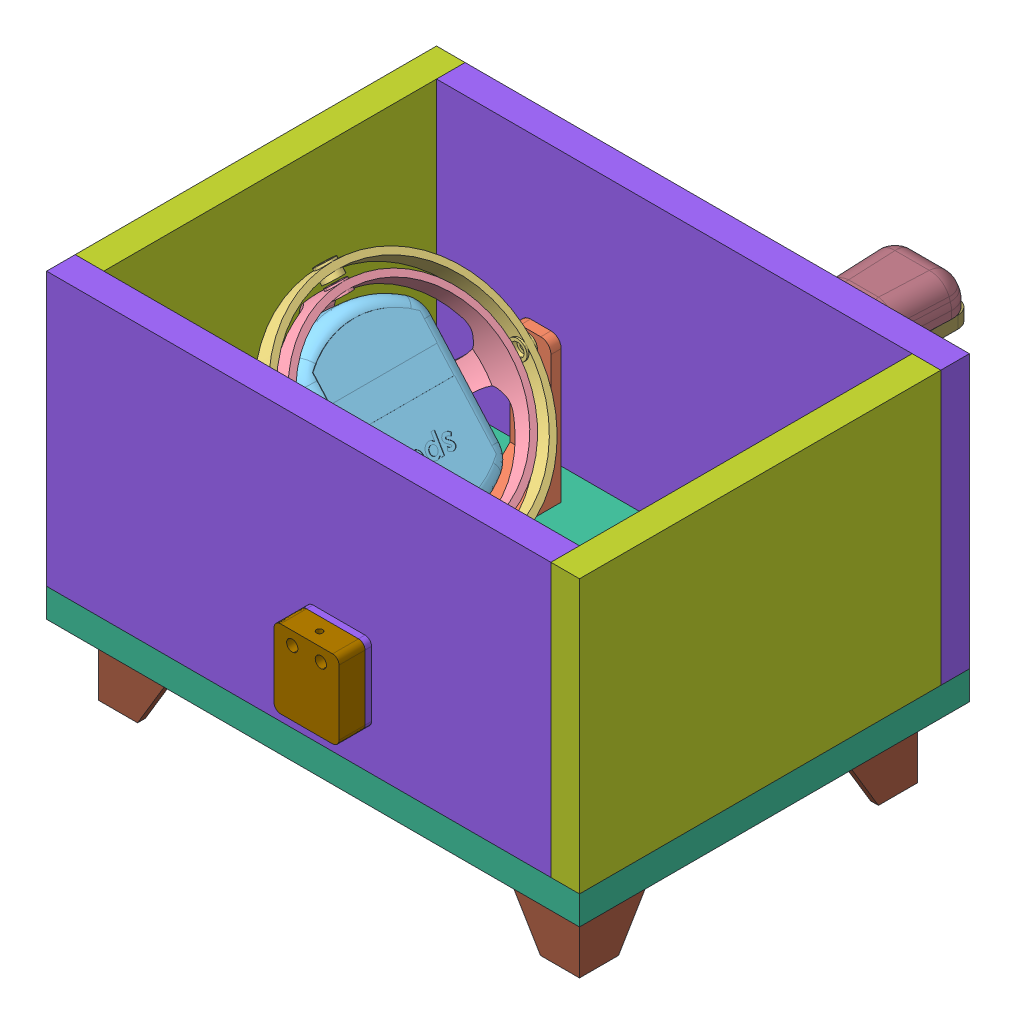
SolidWorks assembly payload_assembly, configuration Default. Lengths in mm.
Overall size (260.35 181.61 252.38).
46 component instances, 33 part files, 70 mates.
Components (placement in the parent):
- arducam_csi_holder-1: arducam_csi_holder [Default] at (27.4723 33.6084 79.928) size (88.89 20 74)
- gyro_outer-1: gyro_outer [Default] at (-22.5277 53.6084 79.928) size (40 70 132)
- gyro_middle-1: gyro_middle [Default] at (-18.9639 122.0052 79.968) x (0 0 1) z (-0.7483 -0.663361 0) size (119.38 119.38 9.62)
- gyro_inner-1: gyro_inner [Default] at (-26.1185 115.7171 79.968) x (0.469068 -0.529127 -0.707107) z (0.469066 -0.529129 0.707107) size (101.6 33.56 101.6)
- SPOT3-1: SPOT3 [Default] at (-41.42 102.8283 80.7299) x (-0.663361 0.7483 0) z (0.000002 0.000002 -1) size (87.12 25.65 65.02)
- payload_bottom-1: payload_bottom [Default] at (27.4723 39.6084 79.928) size (260.35 13.97 190.5)
- payload_front-1: payload_front [Default] at (-102.7027 120.2534 72.943) x (0 0 1) z (0 1 0) size (176.53 13.97 133.35)
- payload_side-5: payload_side [Default] at (20.4873 120.2534 175.178) x (1 0 0) z (0 1 0) size (246.38 13.97 133.35)
- payload_side-6: payload_side [Default] at (34.4573 120.2534 -1.352) x (-1 0 0) z (0 -1 0) size (246.38 13.97 133.35)
- payload_front-2: payload_front [Default] at (157.6473 120.2534 86.913) x (0 0 -1) z (0 1 0) size (176.53 13.97 133.35)
- pi_holder-1: pi_holder [Default] at (34.1673 132.0284 161.208) x (-1 0 0) z (0 0 -1) size (68 59 6)
- RaspberryPi2-1: RaspberryPi2 [Default] at (44.1673 132.0284 153.908) x (1 0 0) z (0 1 0) size (89.62 18.75 58.3)
  - RaspberryPi2 STEP214.STEP-1: RaspberryPi2 STEP214.STEP [Default] at origin size (89.62 18.75 58.3)
    - Mainboard2.STEP-1: Mainboard2.STEP [Default] at origin size (85 1.3 56)
    - GPIO.STEP-1: GPIO.STEP [Default] at (-11.37 0 -24.5) x (0 0 1) z (-1 0 0) size (5 11.5 50.8)
    - Processor.STEP-1: Processor.STEP [Default] at (-15.5 0 -3) x (0 0 1) z (-1 0 0) size (14 1 14)
    - GPU.STEP-1: GPU.STEP [Default] at (15.25 0 -5.75) x (0 0 1) z (-1 0 0) size (9.1 1 9.1)
    - CameraAssembly.STEP-1: CameraAssembly.STEP [Default] at (10.0885 -2.9159 16.55) x (-1 0 0) z (0 0 -1) size (5.01 5.51 22.11)
    - CameraAssembly.STEP-2: CameraAssembly.STEP [Default] at (-46.3885 -2.9159 0) size (5.01 5.51 22.11)
    - HDMI.STEP-1: HDMI.STEP [Default] at (-10.2 0.27 29.3) size (15.04 8.38 12.15)
    - RAM.STEP-1: RAM.STEP [Default] at (0.5 -2.3 -6) x (0 0 1) z (-1 0 0) size (12 1 12)
    - Audio.STEP-1: Audio.STEP [Default] at (10.9 0.15 21.75) size (7 6 14.8)
    - MicroSDSocket.STEP-1: MicroSDSocket.STEP [Default] at (-34.5 -1.3 -0.7) x (0 0 -1) z (-1 0 0) size (13 1.3 14)
    - MicroSD.STEP-1: MicroSD.STEP [Default] at (-37 -2.3 0.1) x (0 0 1) z (-1 0 0) size (11.01 1 15)
    - micro USB2.STEP-1: micro USB2.STEP [Default] at (-17.2704 -5.0969 44.9026) size (7.98 2.93 5.58)
    - usb double.STEP-1: usb double.STEP [Default] at (30.38 -0.09 -18.85) x (0 0 -1) z (1 0 0) size (15.6 18.75 17.92)
    - usb double.STEP-2: usb double.STEP [Default] at (30.38 -0.09 -1.25) x (0 0 -1) z (1 0 0) size (15.6 18.75 17.92)
    - RJ45-LED.STEP-1: RJ45-LED.STEP [Default] at (34.11 7.4 17.348) x (1 0 0) z (0 -1 0) size (21.3 18 14.1)
- qwiik_board-1: qwiik_board [Default] at (33.1823 99.0884 151.408) x (1 0 0) z (0 1 0) size (55 6.08 25)
- Batterie nel portabatterie-1: Batterie nel portabatterie [Default] at (137.5779 63.6178 92.5611) x (0 1 0) z (-1 0 0) size (59.56 61.47 15.11)
  - User Library-R6_AA_UM3-1_5V_holder4AA-2: User Library-R6_AA_UM3-1_5V_holder4AA [4AA] at (18.4086 0.1871 -6.0993) size (59.56 61.47 15.11)
  - Batteria ricaricabile stilo-8: Batteria ricaricabile stilo [Default] at (-4.4514 -22.4504 1.9152) x (0 0 -1) z (1 0 0) size (13.97 13.97 50.04)
  - Batteria ricaricabile stilo-9: Batteria ricaricabile stilo [Default] at (41.2686 -7.3064 2.0287) x (0 0 1) z (-1 0 0) size (13.97 13.97 50.04)
  - Batteria ricaricabile stilo-10: Batteria ricaricabile stilo [Default] at (-4.4514 7.7591 1.9152) x (0 0 -1) z (1 0 0) size (13.97 13.97 50.04)
  - Batteria ricaricabile stilo-11: Batteria ricaricabile stilo [Default] at (-7.4994 22.8246 1.9152) x (0 0 -1) z (1 0 0) size (13.97 13.97 50.04)
- mpl3115a2_altimeter_holder-1: mpl3115a2_altimeter_holder [Default] at (40.1723 91.6784 175.178) x (1 0 0) z (0 -1 0) size (31.75 6.35 38.1)
- mpl3115a2_altimeter_cover-1: mpl3115a2_altimeter_cover [Default] at (40.1723 91.6784 191.053) x (-1 0 0) z (0 -1 0) size (31.75 12.7 38.1)
- arducam_csi-1: arducam_csi [Default] at (27.4723 55.1084 79.928) x (0 0 1) z (1 0 0) size (36 37.5 36)
- leg-1: leg [Default] at (125.8973 39.6084 16.428) x (0 0 1) z (1 0 0) size (38.1 34.29 38.1)
- leg-2: leg [Default] at (125.8973 39.6084 143.428) x (-1 0 0) z (0 0 1) size (38.1 34.29 38.1)
- leg-3: leg [Default] at (-70.9527 39.6084 16.428) x (1 0 0) z (0 0 -1) size (38.1 34.29 38.1)
- leg-4: leg [Default] at (-70.9527 39.6084 143.428) x (0 0 -1) z (-1 0 0) size (38.1 34.29 38.1)
- gps_antenna_holder-1: gps_antenna_holder [Default] at (75.0973 161.5284 -15.322) x (0 -1 0) z (0 0 1) size (34.5 38 46)
- gps_antenna-1: gps_antenna [Default] at (94.318 161.5284 -37.6058) x (0 0 1) z (-1 0 0) size (50 15.5 38.09)
- imu_arduino_holder-1: imu_arduino_holder [Default] at (39.9723 64.6084 68.928) x (1 0 0) z (0 0 -1) size (53 11 56)
- icm20984_imu-1: icm20984_imu [Default] at (52.4723 64.6084 102.928) x (0 0 1) z (-1 0 0) size (26 4.6 26)
Mates (geometry in assembly coordinates):
- Coincident1: coincident anti-aligned: plane of arducam_csi_holder-1 through (27.4723 53.6084 79.928) normal (0 1 0); plane of gyro_outer-1 through (-22.5277 53.6084 79.928) normal (0 -1 0)
- Concentric3: concentric anti-aligned: cylinder of gyro_outer-1 through (-22.5277 118.8459 13.928) axis (0 0 1) radius 1.875; cylinder of gyro_middle-1 through (-22.5277 118.8459 139.658) axis (0 0 -1) radius 1.875
- Distance1: distance = 1.27 mm anti-aligned: plane of gyro_middle-1 through (-14.0453 132.7299 139.658) normal (0 0 1); plane of gyro_outer-1 through (-32.5277 123.6084 140.928) normal (0 0 -1)
- Concentric4: concentric anti-aligned: cylinder of gyro_middle-1 through (-62.1237 163.5119 79.968) axis (0.663361 -0.7483 0) radius 1.875; cylinder of gyro_inner-1 through (25.1034 65.1159 79.968) axis (-0.663361 0.7483 0) radius 1.875
- Distance2: distance = 1.27 mm anti-aligned: plane of gyro_inner-1 through (-71.2246 144.5821 84.7304) normal (-0.663361 0.7483 0); plane of gyro_middle-1 through (-57.5744 158.3801 79.968) normal (0.663361 -0.7483 0)
- Coincident4: coincident anti-aligned: plane of gyro_inner-1 through (-41.0845 102.4499 79.9679) normal (0.7483 0.663361 0.000002); plane of SPOT3-1 through (-44.6011 106.4167 80.7299) normal (-0.7483 -0.663361 -0.000002)
- Distance3: distance = 9.525 mm anti-aligned: plane of SPOT3-1 through (-24.1838 121.6752 54.568) normal (-0.663361 0.7483 0); plane of gyro_inner-1 through (-36.8723 97.6981 130.3695) normal (0.663361 -0.7483 0)
- Distance4: distance = 25.4 mm aligned: plane of SPOT3-1 through (-42.9773 142.8751 48.218) normal (0.000002 0.000002 -1); plane of gyro_inner-1 through (-74.5189 140.1654 73.6179) normal (0.000002 0.000002 -1)
- Coincident10: coincident anti-aligned: plane of arducam_csi_holder-1 through (57.4723 53.6084 109.928) normal (1 0 0); plane of payload_bottom-1 through (57.4723 39.6084 109.928) normal (-1 0 0)
- Coincident11: coincident anti-aligned: plane of arducam_csi_holder-1 through (-2.5277 53.6084 49.928) normal (0 0 -1); plane of payload_bottom-1 through (-2.5277 39.6084 49.928) normal (0 0 1)
- Coincident12: coincident anti-aligned: plane of arducam_csi_holder-1 through (27.4723 39.6084 79.928) normal (0 1 0); plane of payload_bottom-1 through (27.4723 39.6084 79.928) normal (0 -1 0)
- Coincident30: coincident anti-aligned: plane of payload_bottom-1 through (27.4723 53.5784 79.928) normal (0 1 0); plane of payload_front-1 through (-88.7327 53.5784 -15.322) normal (0 -1 0)
- Coincident31: coincident aligned: plane of payload_bottom-1 through (-102.7027 53.5784 -15.322) normal (0 0 -1); plane of payload_front-1 through (-88.7327 186.9284 -15.322) normal (0 0 -1)
- Coincident32: coincident aligned: plane of payload_bottom-1 through (-102.7027 53.5784 175.178) normal (-1 0 0); plane of payload_front-1 through (-102.7027 120.2534 72.943) normal (-1 0 0)
- Coincident33: coincident anti-aligned: plane of payload_front-1 through (-88.7327 186.9284 161.208) normal (0 0 1); plane of payload_side-5 through (20.4873 120.2534 161.208) normal (0 0 -1)
- Coincident34: coincident anti-aligned: plane of payload_bottom-1 through (27.4723 53.5784 79.928) normal (0 1 0); plane of payload_side-5 through (-102.7027 53.5784 161.208) normal (0 -1 0)
- Coincident35: coincident aligned: plane of payload_front-1 through (-102.7027 120.2534 72.943) normal (-1 0 0); plane of payload_side-5 through (-102.7027 186.9284 161.208) normal (-1 0 0)
- Coincident36: coincident anti-aligned: plane of payload_front-1 through (-88.7327 120.2534 72.943) normal (1 0 0); plane of payload_side-6 through (-88.7327 53.5784 -15.322) normal (-1 0 0)
- Coincident37: coincident anti-aligned: plane of payload_bottom-1 through (27.4723 53.5784 79.928) normal (0 1 0); plane of payload_side-6 through (157.6473 53.5784 -15.322) normal (0 -1 0)
- Coincident38: coincident aligned: plane of payload_front-1 through (-88.7327 186.9284 -15.322) normal (0 0 -1); plane of payload_side-6 through (34.4573 120.2534 -15.322) normal (0 0 -1)
- Coincident39: coincident anti-aligned: plane of payload_side-5 through (143.6773 186.9284 161.208) normal (1 0 0); plane of payload_front-2 through (143.6773 120.2534 86.913) normal (-1 0 0)
- Coincident40: coincident anti-aligned: plane of payload_bottom-1 through (27.4723 53.5784 79.928) normal (0 1 0); plane of payload_front-2 through (143.6773 53.5784 175.178) normal (0 -1 0)
- Coincident41: coincident anti-aligned: plane of payload_side-6 through (34.4573 120.2534 -1.352) normal (0 0 1); plane of payload_front-2 through (143.6773 186.9284 -1.352) normal (0 0 -1)
- Coincident42: coincident anti-aligned: plane of payload_side-5 through (20.4873 120.2534 161.208) normal (0 0 -1); plane of pi_holder-1 through (34.1673 132.0284 161.208) normal (0 0 1)
- Concentric13: concentric anti-aligned: cylinder of pi_holder-1 through (63.1673 156.5284 159.208) axis (0 0 1) radius 0.95; cylinder of RaspberryPi2-1/RaspberryPi2 STEP214.STEP-1/Mainboard2.STEP-1 through (63.1673 156.5284 155.208) axis (0 0 -1) radius 1.25
- Parallel4: parallel aligned: plane of pi_holder-1 through (68.1673 161.5284 159.208) normal (0 1 0); plane of RaspberryPi2-1/RaspberryPi2 STEP214.STEP-1/Mainboard2.STEP-1 through (4.1673 160.0284 155.208) normal (0 1 0)
- Coincident46: coincident anti-aligned: plane of pi_holder-1 through (63.1673 156.5284 155.208) normal (0 0 -1); plane of RaspberryPi2-1/RaspberryPi2 STEP214.STEP-1/Mainboard2.STEP-1 through (84.1673 157.5284 155.208) normal (0 0 1)
- Distance7: distance = 25.4 mm aligned: plane of pi_holder-1 through (68.1673 161.5284 159.208) normal (0 1 0); plane of payload_side-5 through (-102.7027 186.9284 161.208) normal (0 1 0)
- Distance8: distance = 88.9 mm anti-aligned: plane of pi_holder-1 through (0.1673 102.5284 159.208) normal (-1 0 0); plane of payload_front-1 through (-88.7327 120.2534 72.943) normal (1 0 0)
- Coincident49: coincident: line of RaspberryPi2-1/RaspberryPi2 STEP214.STEP-1/GPIO.STEP-1 through (9.6873 109.0484 145.508) axis (0 0 1); cylinder of qwiik_board-1 through (9.0523 109.0484 151.408) axis (0 0 -1) radius 0.635
- Coincident50: coincident anti-aligned: plane of RaspberryPi2-1/RaspberryPi2 STEP214.STEP-1/GPIO.STEP-1 through (32.7973 107.5284 151.408) normal (0 0 -1); plane of qwiik_board-1 through (33.1823 99.0884 151.408) normal (0 0 1)
- Coincident51: coincident: line of RaspberryPi2-1/RaspberryPi2 STEP214.STEP-1/GPIO.STEP-1 through (57.9473 109.0484 145.508) axis (0 0 1); cylinder of qwiik_board-1 through (57.3123 109.0484 151.408) axis (0 0 -1) radius 0.635
- Concentric15: concentric aligned: cylinder of mpl3115a2_altimeter_holder-1 through (47.1573 104.3784 175.178) axis (0 0 1) radius 0.95; cylinder of mpl3115a2_altimeter_cover-1 through (47.1573 104.3784 178.353) axis (0 0 1) radius 1.375
- Parallel5: parallel aligned: plane of mpl3115a2_altimeter_holder-1 through (26.9643 75.2954 178.353) normal (-1 0 0); plane of mpl3115a2_altimeter_cover-1 through (24.2973 72.6284 187.878) normal (-1 0 0)
- Coincident60: coincident: plane of mpl3115a2_altimeter_holder-1 through (40.1723 91.6784 178.353) normal (0 0 1); line of mpl3115a2_altimeter_cover-1 through (27.4723 110.7284 178.353) axis (1 0 0)
- Coincident61: coincident anti-aligned: plane of payload_side-5 through (20.4873 120.2534 175.178) normal (0 0 1); plane of mpl3115a2_altimeter_holder-1 through (40.1723 91.6784 175.178) normal (0 0 -1)
- Distance13: distance = 76.2 mm aligned: plane of mpl3115a2_altimeter_cover-1 through (56.0473 110.7284 187.878) normal (0 1 0); plane of payload_side-5 through (-102.7027 186.9284 161.208) normal (0 1 0)
- Distance14: distance = 127 mm aligned: plane of mpl3115a2_altimeter_cover-1 through (24.2973 72.6284 187.878) normal (-1 0 0); plane of payload_side-5 through (-102.7027 186.9284 161.208) normal (-1 0 0)
- Concentric16: concentric anti-aligned: cylinder of arducam_csi_holder-1 through (41.4723 47.6084 65.928) axis (0 1 0) radius 0.95; cylinder of arducam_csi-1 through (41.4723 55.1084 65.928) axis (0 -1 0) radius 1.5
- Concentric17: concentric anti-aligned: cylinder of arducam_csi_holder-1 through (13.4723 47.6084 65.928) axis (0 1 0) radius 0.95; cylinder of arducam_csi-1 through (13.4723 55.1084 65.928) axis (0 -1 0) radius 1.5
- Coincident64: coincident anti-aligned: plane of arducam_csi_holder-1 through (27.4723 53.6084 79.928) normal (0 1 0); plane of arducam_csi-1 through (27.4723 53.6084 79.928) normal (0 -1 0)
- Coincident65: coincident anti-aligned: plane of payload_bottom-1 through (27.4723 39.6084 79.928) normal (0 -1 0); plane of leg-1 through (125.8973 39.6084 16.428) normal (0 1 0)
- Distance15: distance = 12.7 mm aligned: plane of leg-1 through (144.9473 37.0684 -2.622) normal (0 0 -1); plane of payload_bottom-1 through (-102.7027 53.5784 -15.322) normal (0 0 -1)
- Distance16: distance = 12.7 mm aligned: plane of leg-1 through (144.9473 37.0684 -2.622) normal (1 0 0); plane of payload_bottom-1 through (157.6473 53.5784 175.178) normal (1 0 0)
- Coincident68: coincident anti-aligned: plane of payload_bottom-1 through (27.4723 39.6084 79.928) normal (0 -1 0); plane of leg-2 through (125.8973 39.6084 143.428) normal (0 1 0)
- Distance17: distance = 12.7 mm aligned: plane of payload_bottom-1 through (-102.7027 53.5784 175.178) normal (0 0 1); plane of leg-2 through (144.9473 37.0684 162.478) normal (0 0 1)
- Distance18: distance = 12.7 mm aligned: plane of leg-2 through (144.9473 37.0684 162.478) normal (1 0 0); plane of payload_bottom-1 through (157.6473 53.5784 175.178) normal (1 0 0)
- Coincident71: coincident anti-aligned: plane of payload_bottom-1 through (27.4723 39.6084 79.928) normal (0 -1 0); plane of leg-4 through (-70.9527 39.6084 143.428) normal (0 1 0)
- Distance19: distance = 12.7 mm aligned: plane of leg-4 through (-90.0027 37.0684 162.478) normal (-1 0 0); plane of payload_bottom-1 through (-102.7027 53.5784 175.178) normal (-1 0 0)
- Distance20: distance = 12.7 mm aligned: plane of leg-4 through (-90.0027 37.0684 162.478) normal (0 0 1); plane of payload_bottom-1 through (-102.7027 53.5784 175.178) normal (0 0 1)
- Coincident74: coincident anti-aligned: plane of payload_bottom-1 through (27.4723 39.6084 79.928) normal (0 -1 0); plane of leg-3 through (-70.9527 39.6084 16.428) normal (0 1 0)
- Distance22: distance = 12.7 mm aligned: plane of leg-3 through (-90.0027 37.0684 -2.622) normal (0 0 -1); plane of payload_bottom-1 through (-102.7027 53.5784 -15.322) normal (0 0 -1)
- Distance21: distance = 12.7 mm aligned: plane of leg-3 through (-90.0027 37.0684 -2.622) normal (-1 0 0); plane of payload_bottom-1 through (-102.7027 53.5784 175.178) normal (-1 0 0)
- Coincident77: coincident anti-aligned: plane of payload_side-6 through (34.4573 120.2534 -15.322) normal (0 0 -1); plane of gps_antenna_holder-1 through (113.0973 127.0284 -15.322) normal (0 0 1)
- Distance23: distance = 25.4 mm aligned: plane of gps_antenna_holder-1 through (113.0973 161.5284 -15.322) normal (0 1 0); plane of payload_side-6 through (157.6473 186.9284 -15.322) normal (0 1 0)
- Distance24: distance = 177.8 mm aligned: plane of gps_antenna_holder-1 through (75.0973 161.5284 -15.322) normal (-1 0 0); plane of payload_front-1 through (-102.7027 120.2534 72.943) normal (-1 0 0)
- Coincident80: coincident anti-aligned: plane of gps_antenna_holder-1 through (113.0973 161.5284 -15.322) normal (0 1 0); plane of gps_antenna-1 through (94.318 161.5284 -37.6058) normal (0 -1 0)
- Coincident81: coincident aligned: plane of gps_antenna_holder-1 through (113.0973 161.5284 -61.322) normal (0 0 -1); plane of gps_antenna-1 through (74.818 177.0284 -61.322) normal (0 0 -1)
- Distance25: distance = 3.175 mm: line of gps_antenna-1 through (85.2723 161.5284 -61.322) axis (0 1 0); line of gps_antenna_holder-1 through (82.0973 155.5284 -61.322) axis (0 1 0)
- Concentric18: concentric anti-aligned: cylinder of arducam_csi_holder-1 through (2.4723 48.6084 54.928) axis (0 1 0) radius 1.4; cylinder of gyro_outer-1 through (2.4723 119.854 54.928) axis (0 -1 0) radius 1.625
- Concentric19: concentric anti-aligned: cylinder of arducam_csi_holder-1 through (2.4723 48.6084 104.928) axis (0 1 0) radius 1.4; cylinder of gyro_outer-1 through (2.4723 119.854 104.928) axis (0 -1 0) radius 1.625
- Coincident87: coincident anti-aligned: plane of payload_front-2 through (143.6773 120.2534 86.913) normal (-1 0 0); plane of Batterie nel portabatterie-1/User Library-R6_AA_UM3-1_5V_holder4AA-2 through (143.6773 53.5784 123.108) normal (1 0 0)
- Coincident88: coincident anti-aligned: plane of payload_bottom-1 through (27.4723 53.5784 79.928) normal (0 1 0); plane of Batterie nel portabatterie-1/User Library-R6_AA_UM3-1_5V_holder4AA-2 through (128.5643 53.5784 61.64) normal (0 -1 0)
- Distance26: distance = 38.1 mm anti-aligned: plane of Batterie nel portabatterie-1/User Library-R6_AA_UM3-1_5V_holder4AA-2 through (128.5643 53.5784 123.108) normal (0 0 1); plane of payload_side-5 through (20.4873 120.2534 161.208) normal (0 0 -1)
- Concentric20: concentric aligned: cylinder of arducam_csi_holder-1 through (37.4723 48.6084 54.928) axis (0 1 0) radius 1.4; cylinder of imu_arduino_holder-1 through (37.4723 60.6084 54.928) axis (0 1 0) radius 1.875
- Coincident89: coincident anti-aligned: plane of arducam_csi_holder-1 through (27.4723 53.6084 79.928) normal (0 1 0); plane of imu_arduino_holder-1 through (39.9723 53.6084 68.928) normal (0 -1 0)
- Concentric21: concentric aligned: cylinder of arducam_csi_holder-1 through (17.4723 48.6084 54.928) axis (0 1 0) radius 1.4; cylinder of imu_arduino_holder-1 through (17.4723 60.6084 54.928) axis (0 1 0) radius 1.875
- Concentric22: concentric aligned: cylinder of imu_arduino_holder-1 through (62.4723 60.6084 92.928) axis (0 1 0) radius 1.425; cylinder of icm20984_imu-1 through (62.4723 64.6084 92.928) axis (0 1 0) radius 1.625
- Concentric23: concentric aligned: cylinder of imu_arduino_holder-1 through (42.4723 60.6084 92.928) axis (0 1 0) radius 1.425; cylinder of icm20984_imu-1 through (42.4723 64.6084 92.928) axis (0 1 0) radius 1.625
- Coincident90: coincident anti-aligned: plane of imu_arduino_holder-1 through (39.9723 64.6084 68.928) normal (0 1 0); plane of icm20984_imu-1 through (52.4723 64.6084 102.928) normal (0 -1 0)
